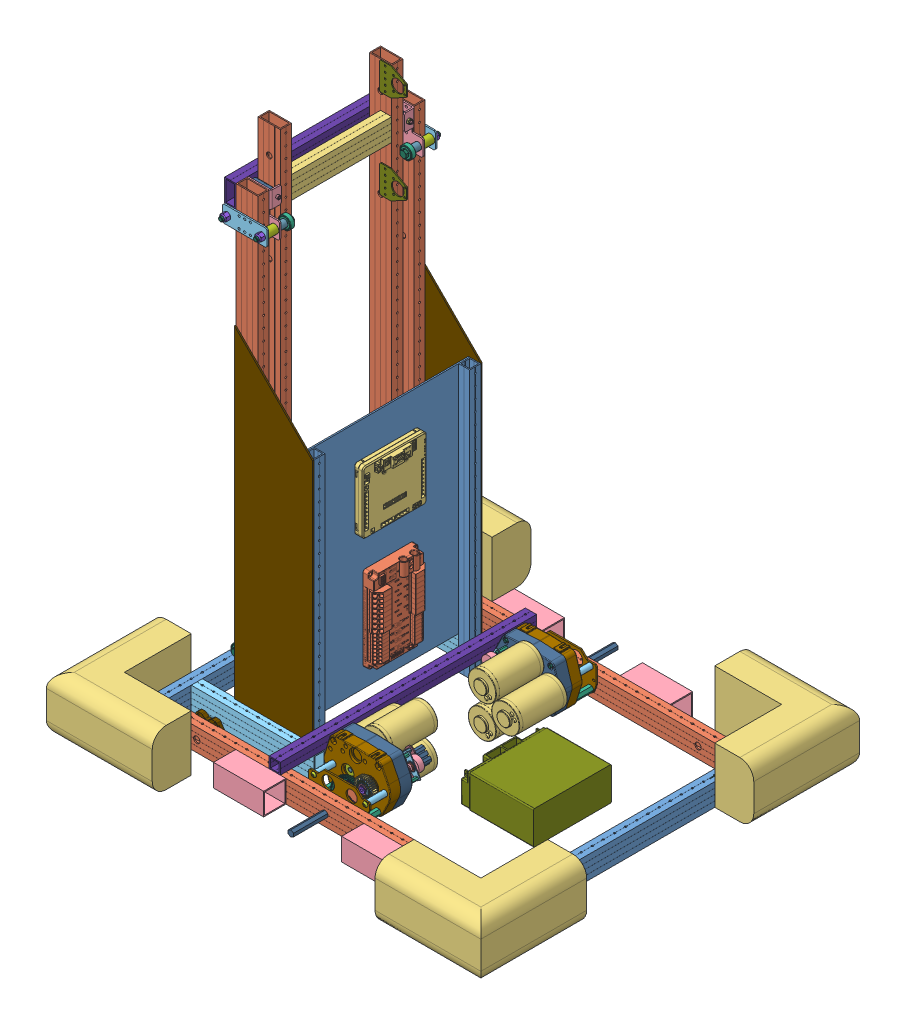
SolidWorks assembly Test Robot 3, configuration Default. Lengths in mm.
Overall size (990.6 1205.52 863.6).
341 component instances, 93 part files, 19 mates.
Components (placement in the parent):
- Test Base 3-1: Test Base 3 [Default] at (-213.2986 -131.6714 217.4582) size (990.6 641.86 863.6)
  - Base Rear Rail-1: Base Rear Rail [Default] at (282.1219 360.9185 104.1623) size (25.4 50.8 685.8)
  - Base Side Rail-1: Base Side Rail [Default] at (1044.1219 360.9185 789.9623) x (0 0 1) z (-1 0 0) size (25.4 50.8 762)
  - Base Side Rail-2: Base Side Rail [Default] at (1044.1219 360.9185 231.1623) x (0 0 1) z (-1 0 0) size (25.4 50.8 762)
  - Blue Bumper-1: Blue Bumper [Default] at (1171.1219 335.5185 942.3623) x (0 0 -1) z (1 0 0) size (241.3 127 241.3)
  - Blue Bumper-2: Blue Bumper [Default] at (1171.1219 335.5185 78.7623) x (-1 0 0) z (0 0 -1) size (241.3 127 241.3)
  - Bumper Support Bar-2: Bumper Support Bar [Default] at (879.0219 335.5185 166.0294) x (0 0 1) z (-1 0 0) size (50.8 50.8 114.3)
  - Bumper Support Bar-4: Bumper Support Bar [Default] at (586.9219 335.5185 166.0294) x (0 0 1) z (-1 0 0) size (50.8 50.8 114.3)
  - Bumper Support Bar-7: Bumper Support Bar [Default] at (586.9219 335.5185 801.0294) x (0 0 1) z (-1 0 0) size (50.8 50.8 114.3)
  - Bumper Support Bar-8: Bumper Support Bar [Default] at (879.0219 335.5185 801.0294) x (0 0 1) z (-1 0 0) size (50.8 50.8 114.3)
  - Base Side Rail Internal-1: Base Side Rail Internal [Default] at (-175.0781 360.9185 713.7623) x (0 0 -1) z (1 0 0) size (25.4 50.8 279.4)
  - Base Side Rail Internal-4: Base Side Rail Internal [Default] at (1044.1219 360.9185 307.3623) x (0 0 1) z (-1 0 0) size (25.4 50.8 279.4)
  - Base Front Rail-1: Base Front Rail [Default] at (1069.5219 360.9185 104.1623) size (25.4 50.8 152.4)
  - 3 CIM Ball Shifter with WCD Output-1: 3 CIM Ball Shifter with WCD Output [Default] at (711.3612 400.7203 682.3171) x (0 1 0) z (0 0 1) size (169.11 183.68 312.65)
    - 217-2733-001 Rev2-1: 217-2733-001 Rev2 [Default] at (0 53.4162 37.6682) x (0 0 1) z (-0.00054 -1 0) size (7.11 24.61 24.61)
    - 217-2733-001 Rev2-2: 217-2733-001 Rev2 [Default] at (0 53.4162 7.9248) x (0 0 -1) z (-0.038475 0.99926 0) size (7.11 24.61 24.61)
    - 217-2731-001 Rev2-1: 217-2731-001 Rev2 [Default] at (0 0 0.0381) x (-0.099212 0.995066 0) z (0.995066 0.099212 0) size (31.12 7.94 31.12)
    - 217-2789-001 Rev2-1: 217-2789-001 Rev2 [Default] at (0 0 43.2943) x (0 0 -1) z (-0.58471 0.811243 0) size (11.1 38.4 38.4)
    - 217-2778-001 Rev2_NCQ8A075-050M_1-1: 217-2778-001 Rev2_NCQ8A075-050M_1 [Default] at (0 0 -53.848) x (-0.707107 0.707107 0) z (0 0 1) size (31.75 33.34 39.88)
      - 217-2778-002_075A-1: 217-2778-002_075A [Default] at origin size (31.75 33.34 26.92)
      - 217-2778-003_075M-1: 217-2778-003_075M [Default] at (0 0 -8.85) x (0.866025 -0.5 0) z (0 0 1) size (18.95 18.95 35.27)
      - 217-2778-004_075-1: 217-2778-004_075 [Default] at (0 0 10.362) size (21 20.74 0.97)
    - 217-2428-012 Rev2-1: 217-2428-012 Rev2 [Default] at (0 0 -40.386) size (63.5 22.23 2.29)
    - 217-2428-005 Rev1-1: 217-2428-005 Rev1 [Default] at (25.4 0 -19.05) x (-0.557362 -0.83027 0) z (-0.83027 0.557362 0) size (7.33 38.98 6.35)
    - 217-2428-005 Rev1-2: 217-2428-005 Rev1 [Default] at (-25.4 0 -19.05) x (0.667436 0.744667 0) z (0.744667 -0.667436 0) size (7.33 38.98 6.35)
    - SCREW-832-0375-1: SCREW-832-0375 [Default] at (25.4 0 -42.5958) x (0 0 1) z (-0.875404 0.483392 0) size (11.73 7.92 7.92)
    - SCREW-832-0375-2: SCREW-832-0375 [Default] at (-25.4 0 -42.5958) x (0 0 1) z (-0.966319 0.257347 0) size (11.73 7.92 7.92)
    - SCREW-832-0375-3: SCREW-832-0375 [Default] at (25.4 0 5.3848) x (0 0 -1) z (1 0 0) size (11.73 7.92 7.92)
    - SCREW-832-0375-4: SCREW-832-0375 [Default] at (-25.4 0 5.3848) x (0 0 -1) z (0.941463 -0.337115 0) size (11.73 7.92 7.92)
    - SBS1_SBS-0632-0250-1: SBS1_SBS-0632-0250 [Default] at (15.494 0 -36.2458) x (0 0 -1) z (0.854303 -0.519775 0) size (8.57 6.68 6.65)
    - SBS1_SBS-0632-0250-2: SBS1_SBS-0632-0250 [Default] at (-15.494 0 -36.2458) x (0 0 -1) z (0.854303 -0.519775 0) size (8.57 6.68 6.65)
    - 217-4098-100 Rev1-1: 217-4098-100 Rev1 [Default] at (0 0 -16.927) x (-0.503316 0.864103 0) z (0 0 1) size (18.03 19.79 22.46)
      - 217-4098-006 Rev2-1: 217-4098-006 Rev2 [Default] at (0 0 -4.6312) x (0 -1 0) z (0 0 -1) size (18.09 11.02 22.46)
      - 217-4098-006 Rev2-2: 217-4098-006 Rev2 [Default] at (0 0 -4.6312) x (0 1 0) z (0 0 -1) size (18.09 11.02 22.46)
      - 217-3489-001 Rev1-1: 217-3489-001 Rev1 [Default] at (0 0 -4.6312) x (0 0 1) z (-0.980217 -0.197926 0) size (4.77 12.7 12.7)
      - 97633A130_97633A130_grv-1: 97633A130_97633A130_grv [Default] at (0 0 -7.33) x (0 0 -1) z (0.979861 0.199683 0) size (0.64 8.74 7.34)
      - 91251A107_91251A107-1: 91251A107_91251A107 [Default] at (-4.8375 -6.735 -9.4343) x (0 0.863883 -0.503692) z (-1 0 0) size (4.65 4.65 10.79)
      - 91251A107_91251A107-2: 91251A107_91251A107 [Default] at (4.8375 6.735 -9.4343) x (0 0.470889 -0.882193) z (1 0 0) size (4.65 4.65 10.79)
    - 217-2428-017 Rev2-1: 217-2428-017 Rev2 [Default] at (12.7 -21.997 -3.614) x (-0.578458 -0.815712 0) z (0 0 -1) size (14.73 14.73 7.37)
    - 217-2428-016 Rev3_Spur01-1: 217-2428-016 Rev3_Spur01 [Default] at (0 0 -3.614) x (0.873157 -0.48744 0) z (0 0 1) size (40.67 40.74 13.32)
    - 217-2428-019 Rev1-1: 217-2428-019 Rev1 [Default] at (12.7 -21.997 -20.6248) x (0.866025 0.5 0) z (0 0 1) size (50.8 19.05 1.57)
    - 217-2428-006 Rev1-1: 217-2428-006 Rev1 [Default] at (32.079 -14.2875 -9.525) x (-0.752416 0.658689 0) z (0.658689 0.752416 0) size (7.33 19.93 6.35)
    - 217-2428-006 Rev1-2: 217-2428-006 Rev1 [Default] at (-3.6662 -34.925 -9.525) x (0.84498 0.534798 0) z (0.534798 -0.84498 0) size (7.33 19.93 6.35)
    - SCREW-832-0375-5: SCREW-832-0375 [Default] at (32.079 -14.2875 4.7498) x (0 0 -1) z (0.980613 0.195955 0) size (11.73 7.92 7.92)
    - SCREW-832-0375-6: SCREW-832-0375 [Default] at (-3.6662 -34.925 5.3848) x (0 0 -1) z (-0.672515 -0.740083 0) size (11.73 7.92 7.92)
    - SCREW-832-0375-7: SCREW-832-0375 [Default] at (-3.6662 -34.925 -22.8346) x (0 0 1) z (0.948865 0.315681 0) size (11.73 7.92 7.92)
    - SCREW-832-0375-8: SCREW-832-0375 [Default] at (32.079 -14.2875 -22.8346) x (0 0 1) z (-0.875404 0.483392 0) size (11.73 7.92 7.92)
    - 217-2614-001_12t-1: 217-2614-001_12t [Default] at (36.9798 39.6868 15.8623) x (-0.087156 0.996195 0) z (0 0 1) size (18.29 18.29 19)
    - 217-2761-001 rev1-1: 217-2761-001 rev1 [Default] at (33.1943 39.3556 16.1) x (0.087156 -0.996195 0) z (0 0 1) size (2 2 20)
    - 217-2761-001 rev1-2: 217-2761-001 rev1 [Default] at (-40.7653 40.018 16.1) x (0.087156 0.996195 0) z (0 0 1) size (2 2 20)
    - 217-2614-001_12t-2: 217-2614-001_12t [Default] at (-36.9798 39.6868 15.8623) x (0.087156 0.996195 0) z (0 0 1) size (18.29 18.29 19)
    - 217-2614-001_12t-3: 217-2614-001_12t [Default] at (0 92.8624 15.8623) x (0.97459 0.223996 0) z (0 0 1) size (18.29 18.29 19)
    - 217-2761-001 rev1-3: 217-2761-001 rev1 [Default] at (-0.8512 96.5658 16.1) x (0.97459 0.223996 0) z (0 0 1) size (2 2 20)
    - 217-3195-002 rev2-1: 217-3195-002 rev2 [Default] at (0 0 50.546) x (-1 0 0) z (0 0 -1) size (114.31 152.24 24.96)
    - 217-3195-001 Rev1-1: 217-3195-001 Rev1 [Default] at origin size (113.41 152.24 26.86)
    - Nylock Nut_NNY2520-ZC-1: Nylock Nut_NNY2520-ZC [Default] at (48.8823 73.025 37.846) x (0 0.866025 -0.5) z (-1 0 0) size (12.85 11.89 7.62)
    - Nylock Nut_NNY2520-ZC-2: Nylock Nut_NNY2520-ZC [Default] at (48.8823 -3.175 37.846) x (0 0 -1) z (-1 0 0) size (12.85 11.89 7.62)
    - Nylock Nut_NNY2520-ZC-3: Nylock Nut_NNY2520-ZC [Default] at (44.45 85.725 7.8613) x (0 1 0) z (0 0 -1) size (12.85 11.89 7.62)
    - 276-1027-001-1: 276-1027-001 [Default] at (47.625 58.1787 6.35) x (0 1 0) z (-1 0 0) size (8.61 5.64 9.94)
    - 276-1027-001-2: 276-1027-001 [Default] at (-47.625 58.1787 6.35) x (0 -1 0) z (1 0 0) size (8.61 5.64 9.94)
    - SCREW-832-1750-1: SCREW-832-1750 [Default] at (-47.625 58.1787 47.0408) x (0 0 -1) z (-0.960822 -0.277167 0) size (46.66 7.92 7.92)
    - SCREW-832-1750-2: SCREW-832-1750 [Default] at (47.625 58.1787 47.0408) x (0 0 -1) z (-0.960822 -0.277167 0) size (46.66 7.92 7.92)
    - Nylock Nut_NNY2520-ZC-4: Nylock Nut_NNY2520-ZC [Default] at (44.45 -15.875 7.8613) x (0 1 0) z (0 0 -1) size (12.85 11.89 7.62)
    - 217-2428-004 Rev3-1: 217-2428-004 Rev3 [Default] at (0 53.4162 22.7711) x (-0.709585 0.70462 0) z (0 0 1) size (11 9.53 43.92)
    - SBS1_SBS-2520-1625SS-1: SBS1_SBS-2520-1625SS [Default] at (44.45 85.725 42.4688) x (0 0 -1) z (-0.251219 0.96793 0) size (45.3 11.2 11.18)
    - SBS1_SBS-2520-1625SS-2: SBS1_SBS-2520-1625SS [Default] at (44.45 -15.875 42.4688) x (0 0 -1) z (-0.251219 0.96793 0) size (45.3 11.2 11.18)
    - SBS1_SBS2520-1750-1: SBS1_SBS2520-1750 [Default] at (-44.45 85.725 7.4422) x (0 0 1) z (-0.031478 0.999504 0) size (48.48 11.22 11.17)
    - SBS1_SBS2520-1750-2: SBS1_SBS2520-1750 [Default] at (-44.45 -15.875 7.4422) x (0 0 1) z (-0.937114 -0.349025 0) size (48.48 11.22 11.17)
    - 217-2428-021 Rev1-1: 217-2428-021 Rev1 [Default] at (0 53.4162 9.5123) x (0.451333 -0.892356 0) z (0 0 1) size (15.88 15.88 3.17)
    - 217-2428-029 Rev1-1: 217-2428-029 Rev1 [Default] at (0 53.4162 36.957) x (0.999846 0.017557 0) z (0 0 1) size (15.88 15.88 1.12)
    - Grayhill Lock Washer-1: Grayhill Lock Washer [Default] at (12.7 -21.997 -18.6817) x (0.467173 -0.884166 0) z (0 0 1) size (19.69 19.69 0.74)
    - Grayhill Nut-1: Grayhill Nut [Default] at (12.7 -21.997 -17.0434) x (0.984088 0.177684 0) z (0 0 1) size (18.33 15.88 2.54)
    - 217-2000-1: 217-2000 [Default] at (0 92.8624 0) x (0 0 -1) z (0.223996 -0.97459 0) size (150.2 64.01 64.01)
    - 217-2000-2: 217-2000 [Default] at (-36.9798 39.6868 0) x (0 0 -1) z (0.996195 -0.087156 0) size (150.2 64.01 64.01)
    - 217-2000-3: 217-2000 [Default] at (36.9798 39.6868 0) x (0 0 -1) z (0.996195 0.087156 0) size (150.2 64.01 64.01)
    - Grahill Encoder-1: Grahill Encoder [Default] at (12.7 -21.997 -16.1798) x (-0.580071 0.814566 0) z (-0.814566 -0.580071 0) size (31.75 31.12 31.75)
    - 217-3195-009 Rev1_wcd 2-1: 217-3195-009 Rev1_wcd 2 [Default] at (0 85.725 50.546) x (-0.998427 -0.056065 0) z (0 0 1) size (12.7 12.7 41.27)
    - 217-3195-006 Rev1_WCD-1: 217-3195-006 Rev1_WCD [Default] at (-44.45 85.725 44.1452) x (0.5 0.866025 0) z (0 0 1) size (12.7 14.66 47.62)
    - 217-3195-009 Rev1_wcd 2-2: 217-3195-009 Rev1_wcd 2 [Default] at (0 -31.75 50.546) x (0.947633 0.319361 0) z (0 0 1) size (12.7 12.7 41.27)
    - 217-3195-006 Rev1_WCD-2: 217-3195-006 Rev1_WCD [Default] at (-44.45 -15.875 44.1452) x (0.5 -0.866025 0) z (0 0 1) size (12.7 14.66 47.62)
    - Nylock Nut_NNY2520-ZC-5: Nylock Nut_NNY2520-ZC [Default] at (0 -31.75 45.0723) x (-0.5 0.866025 0) z (0 0 -1) size (12.85 11.89 7.62)
    - Nylock Nut_NNY2520-ZC-6: Nylock Nut_NNY2520-ZC [Default] at (0 85.725 45.0723) x (-0.5 0.866025 0) z (0 0 -1) size (12.85 11.89 7.62)
    - SBS1_SBS-2520-2250-1: SBS1_SBS-2520-2250 [Default] at (0 -31.75 98.298) x (0 0 -1) z (-0.933488 -0.358607 0) size (61.18 11.22 11.17)
    - SBS1_SBS2520-0625ZC-1: SBS1_SBS2520-0625ZC [Default] at (-44.45 85.725 98.298) x (0 0 -1) z (0.400817 0.916158 0) size (19.57 11.22 11.17)
    - SBS1_SBS2520-0625ZC-2: SBS1_SBS2520-0625ZC [Default] at (-44.45 -15.875 98.298) x (0 0 -1) z (-0.75178 -0.659414 0) size (19.57 11.22 11.17)
    - SBS1_SBS-2520-2250-2: SBS1_SBS-2520-2250 [Default] at (0 85.725 98.298) x (0 0 -1) z (0.056677 -0.998393 0) size (61.18 11.22 11.17)
    - 217-3195-003 rev2-1: 217-3195-003 rev2 [Default] at (0 0 94.9452) size (88.62 139.7 3.17)
    - 217-2617-003 Rev1-1: 217-2617-003 Rev1 [Default] at (-39.878 35.5392 121.8535) x (-0.5 -0.866025 0) z (0 0 1) size (14.66 12.7 152.4)
    - 217-3109-001 Rev1-1: 217-3109-001 Rev1 [Default] at (-39.878 35.5392 49.1808) x (0 0 1) z (0.312889 -0.94979 0) size (7.94 28.57 28.57)
    - 217-2734-001 Rev3-1: 217-2734-001 Rev3 [Default] at (-39.878 35.5392 98.1202) x (1 0 0) z (0 1 0) size (31.12 7.94 31.12)
    - 217-2617-004 Rev1_97431A340_grv-1: 217-2617-004 Rev1_97431A340_grv [Default] at (-39.878 35.5392 54.8961) x (0 0 1) z (-0.124043 -0.992277 0) size (1.07 20.42 18.58)
    - 217-2617-004 Rev1_97431A340_grv-2: 217-2617-004 Rev1_97431A340_grv [Default] at (0 0 69.215) x (0 0 1) z (-0.124043 -0.992277 0) size (1.07 20.42 18.58)
    - 217-2702-001_20t-1: 217-2702-001_20t [Default] at (0 0 62.357) x (0.998435 0.055929 0) z (0 0 1) size (28.2 28.2 12.65)
    - 217-2715-002 Rev1_64t-1: 217-2715-002 Rev1_64t [Default] at (-39.878 35.5392 61.7541) x (0.866025 -0.5 0) z (0 0 1) size (84.3 84.3 12.65)
    - 217-2704-001_24-1: 217-2704-001_24 [Default] at (0 0 62.357) x (0.450781 0.892635 0) z (0 0 -1) size (33.29 33.29 12.65)
    - 217-2714-002 Rev1_60t-1: 217-2714-002 Rev1_60t [Default] at (-39.878 35.5392 61.7541) x (0.866025 -0.5 0) z (0 0 1) size (78.95 78.95 12.65)
    - 217-3221-002 Rev1-1: 217-3221-002 Rev1 [Default] at (-39.878 35.5392 61.7414) x (0 -1 0) z (0 0 1) size (71.39 71.45 12.62)
    - 217-2705-001_30t-1: 217-2705-001_30t [Default] at (0 0 62.357) x (0.547654 -0.836705 0) z (0 0 1) size (41.01 41.12 12.65)
    - 217-2712-002 Rev1_50t-1: 217-2712-002 Rev1_50t [Default] at (-39.878 35.5392 61.7541) x (0.866025 -0.5 0) z (0 0 1) size (66.7 66.76 12.65)
    - 217-2706-001_34t-1: 217-2706-001_34t [Default] at (0 0 62.357) x (0.998435 0.055929 0) z (0 0 1) size (46.46 46.56 12.65)
    - 217-3288-001 Rev3-1: 217-3288-001 Rev3 [Default] at (0 0 0.0889) x (0.055929 -0.998435 0) z (0 0 1) size (99.51 99.53 98.3)
      - 217-2428-008 Rev2-1: 217-2428-008 Rev2 [Default] at (0 0 10.2679) size (31.75 31.75 1.59)
      - 217-2428-028 Rev1_97633A250-1: 217-2428-028 Rev1_97633A250 [Default] at (0 0 37.1221) x (0 0 1) z (0.9357 -0.352797 0) size (1.07 23.39 21.18)
      - 217-4099-000 Rev2_high gear-1: 217-4099-000 Rev2_high gear [Default] x (-1 0 0) z (0 0 1) size (22.23 22.23 98.3)
        - 217-4098-005 Rev1_91612A226-1: 217-4098-005 Rev1_91612A226 [Default] at (0 0 46.2661) x (-0.144757 0 0.989467) z (0 -1 0) size (3.02 3.15 18.22)
        - 217-4098-003 Rev2-1: 217-4098-003 Rev2 [Default] x (1 0 0) z (0 0 -1) size (22.23 22.23 55.94)
        - 217-4099-002 Rev3-1: 217-4099-002 Rev3 [Default] at (0 0 53.467) x (0 0 1) z (-1 0 0) size (40.96 12.73 14.67)
        - 217-4098-004 Rev1-1: 217-4098-004 Rev1 [Default] at (0 0 14.2494) x (0.393904 0.919152 0) z (0 0 1) size (11.68 11.68 56)
      - 217-2428-007 Rev1-1: 217-2428-007 Rev1 [Default] at (7.809 4.5085 14.2494) x (-0.69071 0.455693 -0.561483) z (-0.67559 -0.683536 0.276329) size (6.35 6.35 6.35)
      - 217-2428-007 Rev1-2: 217-2428-007 Rev1 [Default] at (5.4343 3.1375 26.9494) x (-0.162331 -0.978398 0.128005) z (0.857281 -0.204076 -0.472676) size (6.35 6.35 6.35)
      - 217-3212-101 Rev1-1: 217-3212-101 Rev1 [Default] at (-11.5751 10.4131 45.3224) x (0.923728 0.383049 0) z (0 0 -1) size (46.46 46.56 12.7)
        - 217-2428-022 Rev1-1: 217-2428-022 Rev1 [Default] at (6.7035 14.0527 24.6087) size (28.57 28.57 6.1)
        - 217-3212-001 Rev1_34t-1: 217-3212-001 Rev1_34t [Default] at (6.7035 14.0527 27.9107) size (46.46 46.56 11.11)
      - 217-3222-101 Rev1-1: 217-3222-101 Rev1 [Default] at (21.0941 -5.2804 52.7371) x (-0.889163 -0.457591 0) z (0 0 -1) size (73.87 73.92 12.7)
        - 217-2428-022 Rev1-1: 217-2428-022 Rev1 [Default] at (16.3398 14.3476 19.3234) size (28.57 28.57 6.1)
        - 217-3222-001 Rev1_Spur01-1: 217-3222-001 Rev1_Spur01 [Default] at (16.3398 14.3476 22.6254) x (0.999377 0.0353 0) z (0 0 1) size (71.39 71.45 11.11)
      - 217-2428-007 Rev1-3: 217-2428-007 Rev1 [Default] at (-5.4343 3.1375 26.9494) x (0.928483 0.348617 0.128005) z (-0.251905 0.844465 -0.472676) size (6.35 6.35 6.35)
      - 217-2428-007 Rev1-4: 217-2428-007 Rev1 [Default] at (0 -6.275 26.9494) x (-0.766153 0.629782 0.128005) z (-0.605376 -0.640389 -0.472676) size (6.35 6.35 6.35)
      - 217-2428-007 Rev1-5: 217-2428-007 Rev1 [Default] at (-7.809 4.5085 14.2494) x (-0.049287 -0.826019 -0.561483) z (0.929754 -0.24331 0.276329) size (6.35 6.35 6.35)
      - 217-2428-007 Rev1-6: 217-2428-007 Rev1 [Default] at (0 -9.017 14.2494) x (0.739997 0.370326 -0.561483) z (-0.254164 0.926846 0.276329) size (6.35 6.35 6.35)
    - 217-3210-001 Rev1_30t-1: 217-3210-001 Rev1_30t [Default] at (0 53.4162 30.0736) x (-0.966828 0.255427 0) z (0 0 1) size (41.01 41.12 12.65)
    - 217-2711-002 Rev1_50t-1: 217-2711-002 Rev1_50t [Default] at (0 53.4162 17.4244) x (0.262208 -0.965011 0) z (0 0 1) size (66.7 66.76 12.65)
  - 3 CIM Ball Shifter with WCD Output-2: 3 CIM Ball Shifter with WCD Output [Default] at (640.2827 400.7203 338.8075) x (0 1 0) z (0 0 -1) size (169.11 183.68 312.65)
    - 217-2733-001 Rev2-1: 217-2733-001 Rev2 [Default] at (0 53.4162 37.6682) x (0 0 1) z (-0.00054 -1 0) size (7.11 24.61 24.61)
    - 217-2733-001 Rev2-2: 217-2733-001 Rev2 [Default] at (0 53.4162 7.9248) x (0 0 -1) z (-0.038475 0.99926 0) size (7.11 24.61 24.61)
    - 217-2731-001 Rev2-1: 217-2731-001 Rev2 [Default] at (0 0 0.0381) x (-0.099212 0.995066 0) z (0.995066 0.099212 0) size (31.12 7.94 31.12)
    - 217-2789-001 Rev2-1: 217-2789-001 Rev2 [Default] at (0 0 43.2943) x (0 0 -1) z (-0.58471 0.811243 0) size (11.1 38.4 38.4)
    - 217-2778-001 Rev2_NCQ8A075-050M_1-1: 217-2778-001 Rev2_NCQ8A075-050M_1 [Default] at (0 0 -53.848) x (-0.707107 0.707107 0) z (0 0 1) size (31.75 33.34 39.88)
      - 217-2778-002_075A-1: 217-2778-002_075A [Default] at origin size (31.75 33.34 26.92)
      - 217-2778-003_075M-1: 217-2778-003_075M [Default] at (0 0 -8.85) x (0.866025 -0.5 0) z (0 0 1) size (18.95 18.95 35.27)
      - 217-2778-004_075-1: 217-2778-004_075 [Default] at (0 0 10.362) size (21 20.74 0.97)
    - 217-2428-012 Rev2-1: 217-2428-012 Rev2 [Default] at (0 0 -40.386) size (63.5 22.23 2.29)
    - 217-2428-005 Rev1-1: 217-2428-005 Rev1 [Default] at (25.4 0 -19.05) x (-0.557362 -0.83027 0) z (-0.83027 0.557362 0) size (7.33 38.98 6.35)
    - 217-2428-005 Rev1-2: 217-2428-005 Rev1 [Default] at (-25.4 0 -19.05) x (0.667436 0.744667 0) z (0.744667 -0.667436 0) size (7.33 38.98 6.35)
    - SCREW-832-0375-1: SCREW-832-0375 [Default] at (25.4 0 -42.5958) x (0 0 1) z (-0.875404 0.483392 0) size (11.73 7.92 7.92)
    - SCREW-832-0375-2: SCREW-832-0375 [Default] at (-25.4 0 -42.5958) x (0 0 1) z (-0.966319 0.257347 0) size (11.73 7.92 7.92)
    - SCREW-832-0375-3: SCREW-832-0375 [Default] at (25.4 0 5.3848) x (0 0 -1) z (1 0 0) size (11.73 7.92 7.92)
    - SCREW-832-0375-4: SCREW-832-0375 [Default] at (-25.4 0 5.3848) x (0 0 -1) z (0.941463 -0.337115 0) size (11.73 7.92 7.92)
    - SBS1_SBS-0632-0250-1: SBS1_SBS-0632-0250 [Default] at (15.494 0 -36.2458) x (0 0 -1) z (0.854303 -0.519775 0) size (8.57 6.68 6.65)
    - SBS1_SBS-0632-0250-2: SBS1_SBS-0632-0250 [Default] at (-15.494 0 -36.2458) x (0 0 -1) z (0.854303 -0.519775 0) size (8.57 6.68 6.65)
    - 217-4098-100 Rev1-1: 217-4098-100 Rev1 [Default] at (0 0 -16.927) x (-0.503316 0.864103 0) z (0 0 1) size (18.03 19.79 22.46)
      - 217-4098-006 Rev2-1: 217-4098-006 Rev2 [Default] at (0 0 -4.6312) x (0 -1 0) z (0 0 -1) size (18.09 11.02 22.46)
      - 217-4098-006 Rev2-2: 217-4098-006 Rev2 [Default] at (0 0 -4.6312) x (0 1 0) z (0 0 -1) size (18.09 11.02 22.46)
      - 217-3489-001 Rev1-1: 217-3489-001 Rev1 [Default] at (0 0 -4.6312) x (0 0 1) z (-0.980217 -0.197926 0) size (4.77 12.7 12.7)
      - 97633A130_97633A130_grv-1: 97633A130_97633A130_grv [Default] at (0 0 -7.33) x (0 0 -1) z (0.979861 0.199683 0) size (0.64 8.74 7.34)
      - 91251A107_91251A107-1: 91251A107_91251A107 [Default] at (-4.8375 -6.735 -9.4343) x (0 0.863883 -0.503692) z (-1 0 0) size (4.65 4.65 10.79)
      - 91251A107_91251A107-2: 91251A107_91251A107 [Default] at (4.8375 6.735 -9.4343) x (0 0.470889 -0.882193) z (1 0 0) size (4.65 4.65 10.79)
    - 217-2428-017 Rev2-1: 217-2428-017 Rev2 [Default] at (12.7 -21.997 -3.614) x (-0.578458 -0.815712 0) z (0 0 -1) size (14.73 14.73 7.37)
    - 217-2428-016 Rev3_Spur01-1: 217-2428-016 Rev3_Spur01 [Default] at (0 0 -3.614) x (0.873157 -0.48744 0) z (0 0 1) size (40.67 40.74 13.32)
    - 217-2428-019 Rev1-1: 217-2428-019 Rev1 [Default] at (12.7 -21.997 -20.6248) x (0.866025 0.5 0) z (0 0 1) size (50.8 19.05 1.57)
    - 217-2428-006 Rev1-1: 217-2428-006 Rev1 [Default] at (32.079 -14.2875 -9.525) x (-0.752416 0.658689 0) z (0.658689 0.752416 0) size (7.33 19.93 6.35)
    - 217-2428-006 Rev1-2: 217-2428-006 Rev1 [Default] at (-3.6662 -34.925 -9.525) x (0.84498 0.534798 0) z (0.534798 -0.84498 0) size (7.33 19.93 6.35)
    - SCREW-832-0375-5: SCREW-832-0375 [Default] at (32.079 -14.2875 4.7498) x (0 0 -1) z (0.980613 0.195955 0) size (11.73 7.92 7.92)
    - SCREW-832-0375-6: SCREW-832-0375 [Default] at (-3.6662 -34.925 5.3848) x (0 0 -1) z (-0.672515 -0.740083 0) size (11.73 7.92 7.92)
    - SCREW-832-0375-7: SCREW-832-0375 [Default] at (-3.6662 -34.925 -22.8346) x (0 0 1) z (0.948865 0.315681 0) size (11.73 7.92 7.92)
    - SCREW-832-0375-8: SCREW-832-0375 [Default] at (32.079 -14.2875 -22.8346) x (0 0 1) z (-0.875404 0.483392 0) size (11.73 7.92 7.92)
    - 217-2614-001_12t-1: 217-2614-001_12t [Default] at (36.9798 39.6868 15.8623) x (-0.087156 0.996195 0) z (0 0 1) size (18.29 18.29 19)
    - 217-2761-001 rev1-1: 217-2761-001 rev1 [Default] at (33.1943 39.3556 16.1) x (0.087156 -0.996195 0) z (0 0 1) size (2 2 20)
    - 217-2761-001 rev1-2: 217-2761-001 rev1 [Default] at (-40.7653 40.018 16.1) x (0.087156 0.996195 0) z (0 0 1) size (2 2 20)
    - 217-2614-001_12t-2: 217-2614-001_12t [Default] at (-36.9798 39.6868 15.8623) x (0.087156 0.996195 0) z (0 0 1) size (18.29 18.29 19)
    - 217-2614-001_12t-3: 217-2614-001_12t [Default] at (0 92.8624 15.8623) x (0.97459 0.223996 0) z (0 0 1) size (18.29 18.29 19)
    - 217-2761-001 rev1-3: 217-2761-001 rev1 [Default] at (-0.8512 96.5658 16.1) x (0.97459 0.223996 0) z (0 0 1) size (2 2 20)
    - 217-3195-002 rev2-1: 217-3195-002 rev2 [Default] at (0 0 50.546) x (-1 0 0) z (0 0 -1) size (114.31 152.24 24.96)
    - 217-3195-001 Rev1-1: 217-3195-001 Rev1 [Default] at origin size (113.41 152.24 26.86)
    - Nylock Nut_NNY2520-ZC-1: Nylock Nut_NNY2520-ZC [Default] at (48.8823 73.025 37.846) x (0 0.866025 -0.5) z (-1 0 0) size (12.85 11.89 7.62)
    - Nylock Nut_NNY2520-ZC-2: Nylock Nut_NNY2520-ZC [Default] at (48.8823 -3.175 37.846) x (0 0 -1) z (-1 0 0) size (12.85 11.89 7.62)
    - Nylock Nut_NNY2520-ZC-3: Nylock Nut_NNY2520-ZC [Default] at (44.45 85.725 7.8613) x (0 1 0) z (0 0 -1) size (12.85 11.89 7.62)
    - 276-1027-001-1: 276-1027-001 [Default] at (47.625 58.1787 6.35) x (0 1 0) z (-1 0 0) size (8.61 5.64 9.94)
    - 276-1027-001-2: 276-1027-001 [Default] at (-47.625 58.1787 6.35) x (0 -1 0) z (1 0 0) size (8.61 5.64 9.94)
    - SCREW-832-1750-1: SCREW-832-1750 [Default] at (-47.625 58.1787 47.0408) x (0 0 -1) z (-0.960822 -0.277167 0) size (46.66 7.92 7.92)
    - SCREW-832-1750-2: SCREW-832-1750 [Default] at (47.625 58.1787 47.0408) x (0 0 -1) z (-0.960822 -0.277167 0) size (46.66 7.92 7.92)
    - Nylock Nut_NNY2520-ZC-4: Nylock Nut_NNY2520-ZC [Default] at (44.45 -15.875 7.8613) x (0 1 0) z (0 0 -1) size (12.85 11.89 7.62)
    - 217-2428-004 Rev3-1: 217-2428-004 Rev3 [Default] at (0 53.4162 22.7711) x (-0.709585 0.70462 0) z (0 0 1) size (11 9.53 43.92)
    - SBS1_SBS-2520-1625SS-1: SBS1_SBS-2520-1625SS [Default] at (44.45 85.725 42.4688) x (0 0 -1) z (-0.251219 0.96793 0) size (45.3 11.2 11.18)
    - SBS1_SBS-2520-1625SS-2: SBS1_SBS-2520-1625SS [Default] at (44.45 -15.875 42.4688) x (0 0 -1) z (-0.251219 0.96793 0) size (45.3 11.2 11.18)
    - SBS1_SBS2520-1750-1: SBS1_SBS2520-1750 [Default] at (-44.45 85.725 7.4422) x (0 0 1) z (-0.031478 0.999504 0) size (48.48 11.22 11.17)
    - SBS1_SBS2520-1750-2: SBS1_SBS2520-1750 [Default] at (-44.45 -15.875 7.4422) x (0 0 1) z (-0.937114 -0.349025 0) size (48.48 11.22 11.17)
    - 217-2428-021 Rev1-1: 217-2428-021 Rev1 [Default] at (0 53.4162 9.5123) x (0.451333 -0.892356 0) z (0 0 1) size (15.88 15.88 3.17)
    - 217-2428-029 Rev1-1: 217-2428-029 Rev1 [Default] at (0 53.4162 36.957) x (0.999846 0.017557 0) z (0 0 1) size (15.88 15.88 1.12)
    - Grayhill Lock Washer-1: Grayhill Lock Washer [Default] at (12.7 -21.997 -18.6817) x (0.467173 -0.884166 0) z (0 0 1) size (19.69 19.69 0.74)
    - Grayhill Nut-1: Grayhill Nut [Default] at (12.7 -21.997 -17.0434) x (0.984088 0.177684 0) z (0 0 1) size (18.33 15.88 2.54)
    - 217-2000-1: 217-2000 [Default] at (0 92.8624 0) x (0 0 -1) z (0.223996 -0.97459 0) size (150.2 64.01 64.01)
    - 217-2000-2: 217-2000 [Default] at (-36.9798 39.6868 0) x (0 0 -1) z (0.996195 -0.087156 0) size (150.2 64.01 64.01)
    - 217-2000-3: 217-2000 [Default] at (36.9798 39.6868 0) x (0 0 -1) z (0.996195 0.087156 0) size (150.2 64.01 64.01)
    - Grahill Encoder-1: Grahill Encoder [Default] at (12.7 -21.997 -16.1798) x (-0.580071 0.814566 0) z (-0.814566 -0.580071 0) size (31.75 31.12 31.75)
    - 217-3195-009 Rev1_wcd 2-1: 217-3195-009 Rev1_wcd 2 [Default] at (0 85.725 50.546) x (-0.998427 -0.056065 0) z (0 0 1) size (12.7 12.7 41.27)
    - 217-3195-006 Rev1_WCD-1: 217-3195-006 Rev1_WCD [Default] at (-44.45 85.725 44.1452) x (0.5 0.866025 0) z (0 0 1) size (12.7 14.66 47.62)
    - 217-3195-009 Rev1_wcd 2-2: 217-3195-009 Rev1_wcd 2 [Default] at (0 -31.75 50.546) x (0.947633 0.319361 0) z (0 0 1) size (12.7 12.7 41.27)
    - 217-3195-006 Rev1_WCD-2: 217-3195-006 Rev1_WCD [Default] at (-44.45 -15.875 44.1452) x (0.5 -0.866025 0) z (0 0 1) size (12.7 14.66 47.62)
    - Nylock Nut_NNY2520-ZC-5: Nylock Nut_NNY2520-ZC [Default] at (0 -31.75 45.0723) x (-0.5 0.866025 0) z (0 0 -1) size (12.85 11.89 7.62)
    - Nylock Nut_NNY2520-ZC-6: Nylock Nut_NNY2520-ZC [Default] at (0 85.725 45.0723) x (-0.5 0.866025 0) z (0 0 -1) size (12.85 11.89 7.62)
    - SBS1_SBS-2520-2250-1: SBS1_SBS-2520-2250 [Default] at (0 -31.75 98.298) x (0 0 -1) z (-0.933488 -0.358607 0) size (61.18 11.22 11.17)
    - SBS1_SBS2520-0625ZC-1: SBS1_SBS2520-0625ZC [Default] at (-44.45 85.725 98.298) x (0 0 -1) z (0.400817 0.916158 0) size (19.57 11.22 11.17)
    - SBS1_SBS2520-0625ZC-2: SBS1_SBS2520-0625ZC [Default] at (-44.45 -15.875 98.298) x (0 0 -1) z (-0.75178 -0.659414 0) size (19.57 11.22 11.17)
    - SBS1_SBS-2520-2250-2: SBS1_SBS-2520-2250 [Default] at (0 85.725 98.298) x (0 0 -1) z (0.056677 -0.998393 0) size (61.18 11.22 11.17)
    - 217-3195-003 rev2-1: 217-3195-003 rev2 [Default] at (0 0 94.9452) size (88.62 139.7 3.17)
    - 217-2617-003 Rev1-1: 217-2617-003 Rev1 [Default] at (-39.878 35.5392 121.8535) x (-0.5 -0.866025 0) z (0 0 1) size (14.66 12.7 152.4)
    - 217-3109-001 Rev1-1: 217-3109-001 Rev1 [Default] at (-39.878 35.5392 49.1808) x (0 0 1) z (0.312889 -0.94979 0) size (7.94 28.57 28.57)
    - 217-2734-001 Rev3-1: 217-2734-001 Rev3 [Default] at (-39.878 35.5392 98.1202) x (1 0 0) z (0 1 0) size (31.12 7.94 31.12)
    - 217-2617-004 Rev1_97431A340_grv-1: 217-2617-004 Rev1_97431A340_grv [Default] at (-39.878 35.5392 54.8961) x (0 0 1) z (-0.124043 -0.992277 0) size (1.07 20.42 18.58)
    - 217-2617-004 Rev1_97431A340_grv-2: 217-2617-004 Rev1_97431A340_grv [Default] at (0 0 69.215) x (0 0 1) z (-0.124043 -0.992277 0) size (1.07 20.42 18.58)
    - 217-2702-001_20t-1: 217-2702-001_20t [Default] at (0 0 62.357) x (0.998435 0.055929 0) z (0 0 1) size (28.2 28.2 12.65)
    - 217-2715-002 Rev1_64t-1: 217-2715-002 Rev1_64t [Default] at (-39.878 35.5392 61.7541) x (0.866025 -0.5 0) z (0 0 1) size (84.3 84.3 12.65)
    - 217-2704-001_24-1: 217-2704-001_24 [Default] at (0 0 62.357) x (0.450781 0.892635 0) z (0 0 -1) size (33.29 33.29 12.65)
    - 217-2714-002 Rev1_60t-1: 217-2714-002 Rev1_60t [Default] at (-39.878 35.5392 61.7541) x (0.866025 -0.5 0) z (0 0 1) size (78.95 78.95 12.65)
    - 217-3221-002 Rev1-1: 217-3221-002 Rev1 [Default] at (-39.878 35.5392 61.7414) x (0 -1 0) z (0 0 1) size (71.39 71.45 12.62)
    - 217-2705-001_30t-1: 217-2705-001_30t [Default] at (0 0 62.357) x (0.547654 -0.836705 0) z (0 0 1) size (41.01 41.12 12.65)
    - 217-2712-002 Rev1_50t-1: 217-2712-002 Rev1_50t [Default] at (-39.878 35.5392 61.7541) x (0.866025 -0.5 0) z (0 0 1) size (66.7 66.76 12.65)
    - 217-2706-001_34t-1: 217-2706-001_34t [Default] at (0 0 62.357) x (0.998435 0.055929 0) z (0 0 1) size (46.46 46.56 12.65)
    - 217-3288-001 Rev3-1: 217-3288-001 Rev3 [Default] at (0 0 0.0889) x (0.055929 -0.998435 0) z (0 0 1) size (99.51 99.53 98.3)
      - 217-2428-008 Rev2-1: 217-2428-008 Rev2 [Default] at (0 0 10.2679) size (31.75 31.75 1.59)
      - 217-2428-028 Rev1_97633A250-1: 217-2428-028 Rev1_97633A250 [Default] at (0 0 37.1221) x (0 0 1) z (0.9357 -0.352797 0) size (1.07 23.39 21.18)
      - 217-4099-000 Rev2_high gear-1: 217-4099-000 Rev2_high gear [Default] x (-1 0 0) z (0 0 1) size (22.23 22.23 98.3)
        - 217-4098-005 Rev1_91612A226-1: 217-4098-005 Rev1_91612A226 [Default] at (0 0 46.2661) x (-0.144757 0 0.989467) z (0 -1 0) size (3.02 3.15 18.22)
        - 217-4098-003 Rev2-1: 217-4098-003 Rev2 [Default] x (1 0 0) z (0 0 -1) size (22.23 22.23 55.94)
        - 217-4099-002 Rev3-1: 217-4099-002 Rev3 [Default] at (0 0 53.467) x (0 0 1) z (-1 0 0) size (40.96 12.73 14.67)
        - 217-4098-004 Rev1-1: 217-4098-004 Rev1 [Default] at (0 0 14.2494) x (0.393904 0.919152 0) z (0 0 1) size (11.68 11.68 56)
      - 217-2428-007 Rev1-1: 217-2428-007 Rev1 [Default] at (7.809 4.5085 14.2494) x (-0.69071 0.455693 -0.561483) z (-0.67559 -0.683536 0.276329) size (6.35 6.35 6.35)
      - 217-2428-007 Rev1-2: 217-2428-007 Rev1 [Default] at (5.4343 3.1375 26.9494) x (-0.162331 -0.978398 0.128005) z (0.857281 -0.204076 -0.472676) size (6.35 6.35 6.35)
      - 217-3212-101 Rev1-1: 217-3212-101 Rev1 [Default] at (-11.5751 10.4131 45.3224) x (0.923728 0.383049 0) z (0 0 -1) size (46.46 46.56 12.7)
        - 217-2428-022 Rev1-1: 217-2428-022 Rev1 [Default] at (6.7035 14.0527 24.6087) size (28.57 28.57 6.1)
        - 217-3212-001 Rev1_34t-1: 217-3212-001 Rev1_34t [Default] at (6.7035 14.0527 27.9107) size (46.46 46.56 11.11)
      - 217-3222-101 Rev1-1: 217-3222-101 Rev1 [Default] at (21.0941 -5.2804 52.7371) x (-0.889163 -0.457591 0) z (0 0 -1) size (73.87 73.92 12.7)
        - 217-2428-022 Rev1-1: 217-2428-022 Rev1 [Default] at (16.3398 14.3476 19.3234) size (28.57 28.57 6.1)
        - 217-3222-001 Rev1_Spur01-1: 217-3222-001 Rev1_Spur01 [Default] at (16.3398 14.3476 22.6254) x (0.999377 0.0353 0) z (0 0 1) size (71.39 71.45 11.11)
      - 217-2428-007 Rev1-3: 217-2428-007 Rev1 [Default] at (-5.4343 3.1375 26.9494) x (0.928483 0.348617 0.128005) z (-0.251905 0.844465 -0.472676) size (6.35 6.35 6.35)
